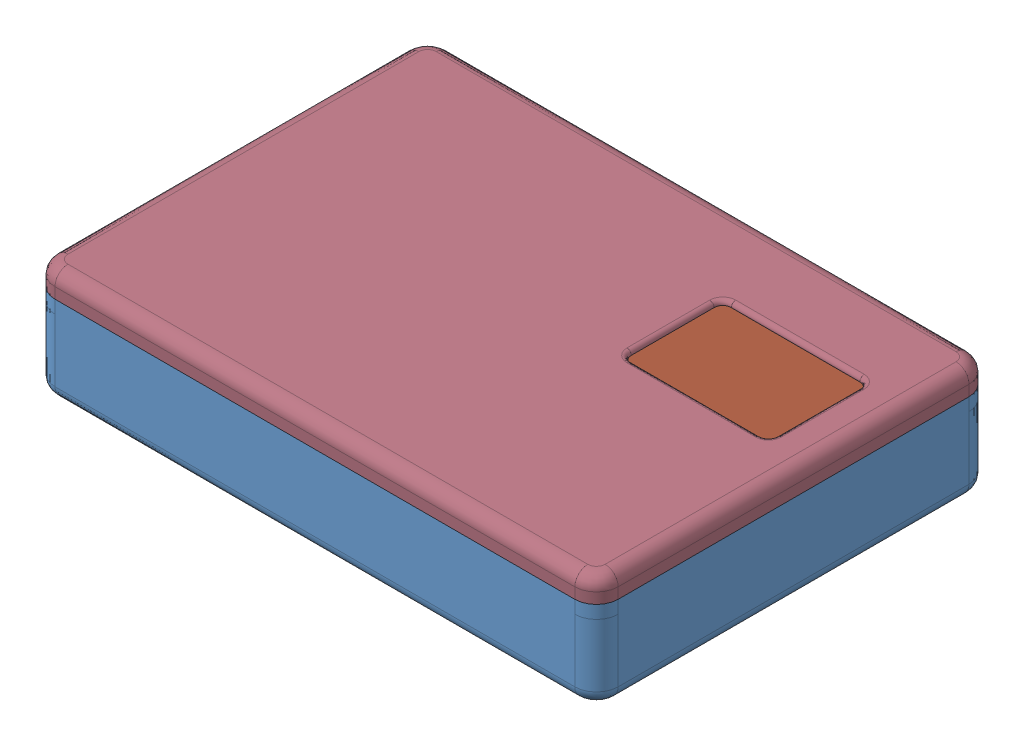
SolidWorks assembly Assembly, configuration Default. Lengths in mm.
Overall size (130.12 26 91.3).
515 component instances, 105 part files, 22 mates.
Components (placement in the parent):
- Part1-1: Part1 [Default] at (-77.6648 36.0917 68.8448) size (130 22.5 91)
- PCB1_2.step-5: PCB1_2.step [Default] at (-142.0534 45.002 144.8645) x (1 0 -0.000465) z (0 1 0) size (68.54 35.94 11.54)
  - Board.step-1: Board.step [Default] at origin size (68.2 35.94 0.41)
    - Open CASCADE STEP translator 7.5 1.1.1.step-1: Open CASCADE STEP translator 7.5 1.1.1.step [Default] at (0 0 -0.4104) size (68.2 35.94 0.41)
  - D6.step-1: D6.step [Default] at origin size (1.3 2.68 1.15)
    - 6259387344.step-1: 6259387344.step [Default] at (99.314 45.339 0) x (0 1 0) z (0 0 1) size (2.67 1.3 1.15)
      - Body.step-1: Body.step [Default] at origin size (1.78 1.3 1.02)
      - FilletPinL.step-1: FilletPinL.step [Default] at origin size (0.45 0.3 0.62)
      - FilletPinR.step-1: FilletPinR.step [Default] at origin size (0.45 0.3 0.62)
  - D5.step-1: D5.step [Default] at origin size (1.3 2.68 1.15)
    - 6259387344.step-1: 6259387344.step [Default] at (97.409 45.466 0) x (0 1 0) z (0 0 1) size (2.67 1.3 1.15)
      - Body.step-1: Body.step [Default] at origin size (1.78 1.3 1.02)
      - FilletPinL.step-1: FilletPinL.step [Default] at origin size (0.45 0.3 0.62)
      - FilletPinR.step-1: FilletPinR.step [Default] at origin size (0.45 0.3 0.62)
  - D4.step-1: D4.step [Default] at origin size (1.3 2.68 1.15)
    - 6259387344.step-1: 6259387344.step [Default] at (75.692 48.387 -0.4104) x (0 -1 0) z (0 0 -1) size (2.67 1.3 1.15)
      - Body.step-1: Body.step [Default] at origin size (1.78 1.3 1.02)
      - FilletPinL.step-1: FilletPinL.step [Default] at origin size (0.45 0.3 0.62)
      - FilletPinR.step-1: FilletPinR.step [Default] at origin size (0.45 0.3 0.62)
  - D3.step-1: D3.step [Default] at origin size (1.3 2.68 1.15)
    - 6259387344.step-1: 6259387344.step [Default] at (75.692 54.356 -0.4104) x (0 -1 0) z (0 0 -1) size (2.67 1.3 1.15)
      - Body.step-1: Body.step [Default] at origin size (1.78 1.3 1.02)
      - FilletPinL.step-1: FilletPinL.step [Default] at origin size (0.45 0.3 0.62)
      - FilletPinR.step-1: FilletPinR.step [Default] at origin size (0.45 0.3 0.62)
  - J3.step-1: J3.step [Default] at origin size (4.01 2 8)
    - Conn_Harwin_M22-2510205_eec.step-1: Conn_Harwin_M22-2510205_eec.step [Default] at (82.931 60.071 0) x (-1 0 0) z (0 0 1) size (4 2 8)
      - Body-0.step-1: Body-0.step [Default] at (-1 0 0.75) x (1 0 0) z (0 -1 0) size (2 1.5 2)
      - Leads.step-1: Leads.step [Default] at (-1 0 0.5) x (-1 0 0) z (0 1 0) size (0.5 8 0.5)
      - Body-0.step-2: Body-0.step [Default] at (1 0 0.75) x (-1 0 0) z (0 1 0) size (2 1.5 2)
      - Leads.step-2: Leads.step [Default] at (1 0 0.5) x (-1 0 0) z (0 1 0) size (0.5 8 0.5)
  - JP3.step-1: JP3.step [Default] at origin size (7.62 2.54 11.54)
    - 61300311121.step-1: 61300311121.step [Default] at (106.0449 39.6239 1.3) x (-1 0 0) z (0 1 0) size (7.62 11.54 2.54)
      - 61300311121-1.step-1: 61300311121-1.step [Default] at origin size (7.62 2.54 2.54)
      - 6130xx11121_PIN.step-1: 6130xx11121_PIN.step [Default] at (-2.54 1.5 0) x (1 0 0) z (0 -1 0) size (0.64 0.64 11.54)
      - 6130xx11121_PIN.step-2: 6130xx11121_PIN.step [Default] at (0 1.5 0) x (1 0 0) z (0 -1 0) size (0.64 0.64 11.54)
      - 6130xx11121_PIN.step-3: 6130xx11121_PIN.step [Default] at (2.54 1.5 0) x (1 0 0) z (0 -1 0) size (0.64 0.64 11.54)
  - R3.step-1: R3.step [Default] at origin size (1.7 0.9 0.55)
    - 6262523328.step-1: 6262523328.step [Default] at (120.381 50.673 0) size (1.2 0.9 0.55)
      - Extruded.step-1: Extruded.step [Default] at origin size (1.2 0.9 0.55)
    - 6262523568.step-1: 6262523568.step [Default] at (119.656 50.673 0) size (0.25 0.9 0.55)
      - Extruded-2.step-1: Extruded-2.step [Default] at origin size (0.25 0.9 0.55)
    - 6262523568.step-2: 6262523568.step [Default] at (121.106 50.673 0) size (0.25 0.9 0.55)
      - Extruded-2.step-1: Extruded-2.step [Default] at origin size (0.25 0.9 0.55)
  - RS1.step-1: RS1.step [Default] at origin size (2.23 3.49 1.16)
    - 6259386784.step-1: 6259386784.step [Default] at (67.945 51.308 -0.4104) x (0 1 0) z (0 0 -1) size (3.49 2.23 1.16)
      - term1.step-1: term1.step [Default] at (-1.6 -0.8 0) size (0.6 1.6 0.65)
      - term2.step-1: term2.step [Default] at (1 -0.8 0) size (0.6 1.6 0.65)
      - Body.step-1: Body.step [Default] at (-1 -0.784 0.0065) size (1.78 1.3 1.02)
  - RNTC1.step-1: RNTC1.step [Default] at origin size (1.6 0.8 0.55)
    - Res_Yageo_RC0603FR-07100KL_eec.step-1: Res_Yageo_RC0603FR-07100KL_eec.step [Default] at (106.4677 42.672 0) x (-1 0 0) z (0 0 1) size (1.6 0.8 0.55)
      - 1.step-1: 1.step [Default] at origin size (1.1 0.8 0.05)
      - 2.step-1: 2.step [Default] at origin size (1.5 0.8 0.45)
      - 3.step-1: 3.step [Default] at origin size (1.6 0.8 0.55)
      - Yageo Logo.step-1: Yageo Logo.step [Default] at (-1.8829 0.0903 0.5401) size (0.34 0.08 0.01)
  - R5.step-1: R5.step [Default] at origin size (1.6 0.8 0.55)
    - 6259379744.step-1: 6259379744.step [Default] at (80.379 48.006 0) x (-1 0 0) z (0 0 1) size (1.6 0.8 0.55)
      - term1-3.step-1: term1-3.step [Default] at (-0.8 -0.4 0) size (0.25 0.8 0.55)
      - term2-4.step-1: term2-4.step [Default] at (0.55 -0.4 0) size (0.25 0.8 0.55)
      - body-5.step-1: body-5.step [Default] at (-0.55 -0.392 0.0055) size (1.1 0.78 0.54)
  - R32.step-1: R32.step [Default] at origin size (2.5 5 0.55)
    - 6151998672.step-1: 6151998672.step [Default] at (98.688 58.674 0) size (2.5 5 0.55)
      - solidBody.step-1: solidBody.step [Default] at origin size (2.4 5 0.45)
      - Terminal.step-1: Terminal.step [Default] at origin size (2.5 5 0.54)
      - solidTop.step-1: solidTop.step [Default] at origin size (1.8 4.9 0.05)
  - R31.step-1: R31.step [Default] at origin size (1.6 0.8 0.55)
    - 6259379744.step-1: 6259379744.step [Default] at (102.87 44.069 0) x (-1 0 0) z (0 0 1) size (1.6 0.8 0.55)
      - term1-3.step-1: term1-3.step [Default] at (-0.8 -0.4 0) size (0.25 0.8 0.55)
      - term2-4.step-1: term2-4.step [Default] at (0.55 -0.4 0) size (0.25 0.8 0.55)
      - body-5.step-1: body-5.step [Default] at (-0.55 -0.392 0.0055) size (1.1 0.78 0.54)
  - R30.step-1: R30.step [Default] at origin size (0.9 1.7 0.55)
    - 6262524208.step-1: 6262524208.step [Default] at (103.124 48.002 0) size (0.9 1.2 0.55)
      - Extruded-6.step-1: Extruded-6.step [Default] at origin size (0.9 1.2 0.55)
    - 6262524048.step-1: 6262524048.step [Default] at (103.124 47.277 0) size (0.9 0.25 0.55)
      - Extruded-7.step-1: Extruded-7.step [Default] at origin size (0.9 0.25 0.55)
    - 6262524048.step-2: 6262524048.step [Default] at (103.124 48.727 0) size (0.9 0.25 0.55)
      - Extruded-7.step-1: Extruded-7.step [Default] at origin size (0.9 0.25 0.55)
  - R29.step-1: R29.step [Default] at origin size (0.8 1.6 0.55)
    - 6259384304.step-1: 6259384304.step [Default] at (111.252 42.168 0) x (0 1 0) z (0 0 1) size (1.6 0.8 0.55)
      - term1-8.step-1: term1-8.step [Default] at (-0.8 -0.4 0) size (0.25 0.8 0.55)
      - term2-9.step-1: term2-9.step [Default] at (0.55 -0.4 0) size (0.25 0.8 0.55)
      - body-10.step-1: body-10.step [Default] at (-0.55 -0.392 0.0055) size (1.1 0.78 0.54)
  - R27.step-1: R27.step [Default] at origin size (0.8 1.6 0.55)
    - 6259384304.step-1: 6259384304.step [Default] at (106.426 45.428 0) x (0 1 0) z (0 0 1) size (1.6 0.8 0.55)
      - term1-8.step-1: term1-8.step [Default] at (-0.8 -0.4 0) size (0.25 0.8 0.55)
      - term2-9.step-1: term2-9.step [Default] at (0.55 -0.4 0) size (0.25 0.8 0.55)
      - body-10.step-1: body-10.step [Default] at (-0.55 -0.392 0.0055) size (1.1 0.78 0.54)
  - R26.step-1: R26.step [Default] at origin size (0.9 1.7 0.55)
    - 6262524208.step-1: 6262524208.step [Default] at (107.823 45.72 0) size (0.9 1.2 0.55)
      - Extruded-6.step-1: Extruded-6.step [Default] at origin size (0.9 1.2 0.55)
    - 6262524048.step-1: 6262524048.step [Default] at (107.823 44.995 0) size (0.9 0.25 0.55)
      - Extruded-7.step-1: Extruded-7.step [Default] at origin size (0.9 0.25 0.55)
    - 6262524048.step-2: 6262524048.step [Default] at (107.823 46.445 0) size (0.9 0.25 0.55)
      - Extruded-7.step-1: Extruded-7.step [Default] at origin size (0.9 0.25 0.55)
  - R25.step-1: R25.step [Default] at origin size (0.8 1.6 0.55)
    - 6259384304.step-1: 6259384304.step [Default] at (101.854 47.752 0) x (0 1 0) z (0 0 1) size (1.6 0.8 0.55)
      - term1-8.step-1: term1-8.step [Default] at (-0.8 -0.4 0) size (0.25 0.8 0.55)
      - term2-9.step-1: term2-9.step [Default] at (0.55 -0.4 0) size (0.25 0.8 0.55)
      - body-10.step-1: body-10.step [Default] at (-0.55 -0.392 0.0055) size (1.1 0.78 0.54)
  - R24.step-1: R24.step [Default] at origin size (1.6 0.8 0.55)
    - 6151993232.step-1: 6151993232.step [Default] at (94.615 46.609 0) size (1.6 0.8 0.55)
      - term1-11.step-1: term1-11.step [Default] at (-0.8 -0.4 0) size (0.25 0.8 0.55)
      - term2-12.step-1: term2-12.step [Default] at (0.55 -0.4 0) size (0.25 0.8 0.55)
      - body-13.step-1: body-13.step [Default] at (-0.55 -0.392 0.0055) size (1.1 0.78 0.54)
  - R23.step-1: R23.step [Default] at origin size (1.6 0.8 0.55)
    - 6259379744.step-1: 6259379744.step [Default] at (80.379 46.228 0) x (-1 0 0) z (0 0 1) size (1.6 0.8 0.55)
      - term1-3.step-1: term1-3.step [Default] at (-0.8 -0.4 0) size (0.25 0.8 0.55)
      - term2-4.step-1: term2-4.step [Default] at (0.55 -0.4 0) size (0.25 0.8 0.55)
      - body-5.step-1: body-5.step [Default] at (-0.55 -0.392 0.0055) size (1.1 0.78 0.54)
  - R22.step-1: R22.step [Default] at origin size (1.7 0.9 0.55)
    - 6262523568.step-1: 6262523568.step [Default] at (107.659 48.387 0) size (0.25 0.9 0.55)
      - Extruded-2.step-1: Extruded-2.step [Default] at origin size (0.25 0.9 0.55)
    - 6262523568.step-2: 6262523568.step [Default] at (106.209 48.387 0) size (0.25 0.9 0.55)
      - Extruded-2.step-1: Extruded-2.step [Default] at origin size (0.25 0.9 0.55)
    - 6262523328.step-1: 6262523328.step [Default] at (106.934 48.387 0) size (1.2 0.9 0.55)
      - Extruded.step-1: Extruded.step [Default] at origin size (1.2 0.9 0.55)
  - R21.step-1: R21.step [Default] at origin size (0.9 1.7 0.55)
    - 6262524208.step-1: 6262524208.step [Default] at (109.474 42.418 0) size (0.9 1.2 0.55)
      - Extruded-6.step-1: Extruded-6.step [Default] at origin size (0.9 1.2 0.55)
    - 6262524048.step-1: 6262524048.step [Default] at (109.474 43.143 0) size (0.9 0.25 0.55)
      - Extruded-7.step-1: Extruded-7.step [Default] at origin size (0.9 0.25 0.55)
    - 6262524048.step-2: 6262524048.step [Default] at (109.474 41.693 0) size (0.9 0.25 0.55)
      - Extruded-7.step-1: Extruded-7.step [Default] at origin size (0.9 0.25 0.55)
  - R20.step-1: R20.step [Default] at origin size (1.6 0.8 0.55)
    - 6259388464.step-1: 6259388464.step [Default] at (94.615 48.006 0) x (1 0 0) z (0 0 1) size (1.6 0.8 0.55)
      - term1-14.step-1: term1-14.step [Default] at (-0.8 -0.4 0) size (0.25 0.8 0.55)
      - term2-15.step-1: term2-15.step [Default] at (0.55 -0.4 0) size (0.25 0.8 0.55)
      - body-16.step-1: body-16.step [Default] at (-0.55 -0.392 0.0055) size (1.1 0.78 0.54)
  - R19.step-1: R19.step [Default] at origin size (0.8 1.6 0.55)
    - 6259384304.step-1: 6259384304.step [Default] at (104.648 47.752 0) x (0 1 0) z (0 0 1) size (1.6 0.8 0.55)
      - term1-8.step-1: term1-8.step [Default] at (-0.8 -0.4 0) size (0.25 0.8 0.55)
      - term2-9.step-1: term2-9.step [Default] at (0.55 -0.4 0) size (0.25 0.8 0.55)
      - body-10.step-1: body-10.step [Default] at (-0.55 -0.392 0.0055) size (1.1 0.78 0.54)
  - R18.step-1: R18.step [Default] at origin size (1.7 0.9 0.55)
    - 6262523328.step-1: 6262523328.step [Default] at (94.615 49.276 0) size (1.2 0.9 0.55)
      - Extruded.step-1: Extruded.step [Default] at origin size (1.2 0.9 0.55)
    - 6262523568.step-1: 6262523568.step [Default] at (93.89 49.276 0) size (0.25 0.9 0.55)
      - Extruded-2.step-1: Extruded-2.step [Default] at origin size (0.25 0.9 0.55)
    - 6262523568.step-2: 6262523568.step [Default] at (95.34 49.276 0) size (0.25 0.9 0.55)
      - Extruded-2.step-1: Extruded-2.step [Default] at origin size (0.25 0.9 0.55)
  - R17.step-1: R17.step [Default] at origin size (1.6 0.8 0.55)
    - Res_Yageo_RC0603FR-07100KL_eec.step-1: Res_Yageo_RC0603FR-07100KL_eec.step [Default] at (94.615 50.8 0) size (1.6 0.8 0.55)
      - 1.step-1: 1.step [Default] at origin size (1.1 0.8 0.05)
      - 2.step-1: 2.step [Default] at origin size (1.5 0.8 0.45)
      - 3.step-1: 3.step [Default] at origin size (1.6 0.8 0.55)
      - Yageo Logo.step-1: Yageo Logo.step [Default] at (-1.8829 0.0903 0.5401) size (0.34 0.08 0.01)
  - R16.step-1: R16.step [Default] at origin size (1.6 0.8 0.55)
    - 6259379744.step-1: 6259379744.step [Default] at (115.443 54.102 0) x (-1 0 0) z (0 0 1) size (1.6 0.8 0.55)
      - term1-3.step-1: term1-3.step [Default] at (-0.8 -0.4 0) size (0.25 0.8 0.55)
      - term2-4.step-1: term2-4.step [Default] at (0.55 -0.4 0) size (0.25 0.8 0.55)
      - body-5.step-1: body-5.step [Default] at (-0.55 -0.392 0.0055) size (1.1 0.78 0.54)
  - R15.step-1: R15.step [Default] at origin size (2.5 5 0.55)
    - 6151998672.step-1: 6151998672.step [Default] at (94.488 58.547 0) size (2.5 5 0.55)
      - solidBody.step-1: solidBody.step [Default] at origin size (2.4 5 0.45)
      - Terminal.step-1: Terminal.step [Default] at origin size (2.5 5 0.54)
      - solidTop.step-1: solidTop.step [Default] at origin size (1.8 4.9 0.05)
  - R14.step-1: R14.step [Default] at origin size (1.7 0.9 0.55)
    - 6262523568.step-1: 6262523568.step [Default] at (85.561 51.943 0) size (0.25 0.9 0.55)
      - Extruded-2.step-1: Extruded-2.step [Default] at origin size (0.25 0.9 0.55)
    - 6262523568.step-2: 6262523568.step [Default] at (84.111 51.943 0) size (0.25 0.9 0.55)
      - Extruded-2.step-1: Extruded-2.step [Default] at origin size (0.25 0.9 0.55)
    - 6262523328.step-1: 6262523328.step [Default] at (84.836 51.943 0) size (1.2 0.9 0.55)
      - Extruded.step-1: Extruded.step [Default] at origin size (1.2 0.9 0.55)
  - R13.step-1: R13.step [Default] at origin size (2.5 5 0.55)
    - 6151998672.step-1: 6151998672.step [Default] at (126.365 58.928 0) size (2.5 5 0.55)
      - solidBody.step-1: solidBody.step [Default] at origin size (2.4 5 0.45)
      - Terminal.step-1: Terminal.step [Default] at origin size (2.5 5 0.54)
      - solidTop.step-1: solidTop.step [Default] at origin size (1.8 4.9 0.05)
  - R12.step-1: R12.step [Default] at origin size (2.5 5 0.55)
    - 6151998672.step-1: 6151998672.step [Default] at (122.174 58.928 0) size (2.5 5 0.55)
      - solidBody.step-1: solidBody.step [Default] at origin size (2.4 5 0.45)
      - Terminal.step-1: Terminal.step [Default] at origin size (2.5 5 0.54)
      - solidTop.step-1: solidTop.step [Default] at origin size (1.8 4.9 0.05)
  - R11.step-1: R11.step [Default] at origin size (1.6 0.8 0.55)
    - 6259379744.step-1: 6259379744.step [Default] at (94.5879 54.102 0) x (-1 0 0) z (0 0 1) size (1.6 0.8 0.55)
      - term1-3.step-1: term1-3.step [Default] at (-0.8 -0.4 0) size (0.25 0.8 0.55)
      - term2-4.step-1: term2-4.step [Default] at (0.55 -0.4 0) size (0.25 0.8 0.55)
      - body-5.step-1: body-5.step [Default] at (-0.55 -0.392 0.0055) size (1.1 0.78 0.54)
  - R10.step-1: R10.step [Default] at origin size (1.6 0.8 0.55)
    - 6259379744.step-1: 6259379744.step [Default] at (94.5879 52.451 0) x (-1 0 0) z (0 0 1) size (1.6 0.8 0.55)
      - term1-3.step-1: term1-3.step [Default] at (-0.8 -0.4 0) size (0.25 0.8 0.55)
      - term2-4.step-1: term2-4.step [Default] at (0.55 -0.4 0) size (0.25 0.8 0.55)
      - body-5.step-1: body-5.step [Default] at (-0.55 -0.392 0.0055) size (1.1 0.78 0.54)
  - R9.step-1: R9.step [Default] at origin size (1.6 0.8 0.55)
    - 6151993232.step-1: 6151993232.step [Default] at (115.443 55.753 0) size (1.6 0.8 0.55)
      - term1-11.step-1: term1-11.step [Default] at (-0.8 -0.4 0) size (0.25 0.8 0.55)
      - term2-12.step-1: term2-12.step [Default] at (0.55 -0.4 0) size (0.25 0.8 0.55)
      - body-13.step-1: body-13.step [Default] at (-0.55 -0.392 0.0055) size (1.1 0.78 0.54)
  - R8.step-1: R8.step [Default] at origin size (0.8 1.6 0.55)
    - 6259393184.step-1: 6259393184.step [Default] at (118.237 62.23 0) x (0 -1 0) z (0 0 1) size (1.6 0.8 0.55)
      - term1-17.step-1: term1-17.step [Default] at (-0.8 -0.4 0) size (0.25 0.8 0.55)
      - term2-18.step-1: term2-18.step [Default] at (0.55 -0.4 0) size (0.25 0.8 0.55)
      - body-19.step-1: body-19.step [Default] at (-0.55 -0.392 0.0055) size (1.1 0.78 0.54)
  - R7.step-1: R7.step [Default] at origin size (0.8 1.6 0.55)
    - 6259384304.step-1: 6259384304.step [Default] at (109.728 62.268 0) x (0 1 0) z (0 0 1) size (1.6 0.8 0.55)
      - term1-8.step-1: term1-8.step [Default] at (-0.8 -0.4 0) size (0.25 0.8 0.55)
      - term2-9.step-1: term2-9.step [Default] at (0.55 -0.4 0) size (0.25 0.8 0.55)
      - body-10.step-1: body-10.step [Default] at (-0.55 -0.392 0.0055) size (1.1 0.78 0.54)
  - R6.step-1: R6.step [Default] at origin size (0.8 1.6 0.55)
    - 6259393184.step-1: 6259393184.step [Default] at (90.551 48.73 0) x (0 -1 0) z (0 0 1) size (1.6 0.8 0.55)
      - term1-17.step-1: term1-17.step [Default] at (-0.8 -0.4 0) size (0.25 0.8 0.55)
      - term2-18.step-1: term2-18.step [Default] at (0.55 -0.4 0) size (0.25 0.8 0.55)
      - body-19.step-1: body-19.step [Default] at (-0.55 -0.392 0.0055) size (1.1 0.78 0.54)
  - R4.step-1: R4.step [Default] at origin size (1.7 0.9 0.55)
    - 6262523568.step-1: 6262523568.step [Default] at (125.17 46.101 0) size (0.25 0.9 0.55)
      - Extruded-2.step-1: Extruded-2.step [Default] at origin size (0.25 0.9 0.55)
    - 6262523568.step-2: 6262523568.step [Default] at (123.72 46.101 0) size (0.25 0.9 0.55)
      - Extruded-2.step-1: Extruded-2.step [Default] at origin size (0.25 0.9 0.55)
    - 6262523328.step-1: 6262523328.step [Default] at (124.445 46.101 0) size (1.2 0.9 0.55)
      - Extruded.step-1: Extruded.step [Default] at origin size (1.2 0.9 0.55)
  - R2.step-1: R2.step [Default] at origin size (1.6 0.8 0.55)
    - 6259379744.step-1: 6259379744.step [Default] at (124.549 47.752 0) x (-1 0 0) z (0 0 1) size (1.6 0.8 0.55)
      - term1-3.step-1: term1-3.step [Default] at (-0.8 -0.4 0) size (0.25 0.8 0.55)
      - term2-4.step-1: term2-4.step [Default] at (0.55 -0.4 0) size (0.25 0.8 0.55)
      - body-5.step-1: body-5.step [Default] at (-0.55 -0.392 0.0055) size (1.1 0.78 0.54)
  - R1.step-1: R1.step [Default] at origin size (0.8 1.6 0.55)
    - 6259384304.step-1: 6259384304.step [Default] at (118.872 53.213 0) x (0 1 0) z (0 0 1) size (1.6 0.8 0.55)
      - term1-8.step-1: term1-8.step [Default] at (-0.8 -0.4 0) size (0.25 0.8 0.55)
      - term2-9.step-1: term2-9.step [Default] at (0.55 -0.4 0) size (0.25 0.8 0.55)
      - body-10.step-1: body-10.step [Default] at (-0.55 -0.392 0.0055) size (1.1 0.78 0.54)
  - P2.step-1: P2.step [Default] at origin size (12.7 2.54 11.54)
    - 61300511121.step-1: 61300511121.step [Default] at (94.2339 39.7509 1.3) x (-1 0 0) z (0 1 0) size (12.7 11.54 2.54)
      - 6130xx11121_PIN-20.step-1: 6130xx11121_PIN-20.step [Default] at (-5.08 1.5 0) x (1 0 0) z (0 -1 0) size (0.64 0.64 11.54)
      - 6130xx11121_PIN-20.step-2: 6130xx11121_PIN-20.step [Default] at (-2.54 1.5 0) x (1 0 0) z (0 -1 0) size (0.64 0.64 11.54)
      - 6130xx11121_PIN-20.step-3: 6130xx11121_PIN-20.step [Default] at (0 1.5 0) x (1 0 0) z (0 -1 0) size (0.64 0.64 11.54)
      - 6130xx11121_PIN-20.step-4: 6130xx11121_PIN-20.step [Default] at (2.54 1.5 0) x (1 0 0) z (0 -1 0) size (0.64 0.64 11.54)
      - 6130xx11121_PIN-20.step-5: 6130xx11121_PIN-20.step [Default] at (5.08 1.5 0) x (1 0 0) z (0 -1 0) size (0.64 0.64 11.54)
      - 61300511121-21.step-1: 61300511121-21.step [Default] at origin size (12.7 2.54 2.54)
  - P1.step-1: P1.step [Default] at origin size (10.49 9.2 5.39)
    - 6259392944.step-1: 6259392944.step [Default] at (64.299 51.054 1.59) x (-1 0 0) z (0 0 1) size (10.49 9.2 5.39)
  - M2.step-1: M2.step [Default] at origin size (3.3 3.3 1.06)
    - 6259390624.step-1: 6259390624.step [Default] at (88.799 55.336 0.02) x (-1 0 0) z (0 1 0) size (3.3 1.06 3.3)
  - M1.step-1: M1.step [Default] at origin size (3.3 3.3 1.06)
    - 6259390624.step-1: 6259390624.step [Default] at (84.709 55.246 0.02) x (-1 0 0) z (0 1 0) size (3.3 1.06 3.3)
  - LED1.step-1: LED1.step [Default] at origin size (1 2 0.7)
    - 6259379424.step-1: 6259379424.step [Default] at (110.774 46.833 0.12) x (0 -1 0) z (-1 0 0) size (2 0.7 1)
  - L1.step-1: L1.step [Default] at origin size (4 4 3.1)
    - 6151993152.step-1: 6151993152.step [Default] at (113.919 60.579 0) size (4 4 3.1)
      - Body-22.step-1: Body-22.step [Default] at (0 0 0.1) size (4 4 3)
      - Pins.step-1: Pins.step [Default] at origin size (3.87 3.37 0.1)
  - JP2.step-1: JP2.step [Default] at origin size (7.62 2.54 11.54)
    - 61300311121.step-1: 61300311121.step [Default] at (117.0941 41.5291 1.3) x (1 0 0) z (0 -1 0) size (7.62 11.54 2.54)
      - 61300311121-1.step-1: 61300311121-1.step [Default] at origin size (7.62 2.54 2.54)
      - 6130xx11121_PIN.step-1: 6130xx11121_PIN.step [Default] at (-2.54 1.5 0) x (1 0 0) z (0 -1 0) size (0.64 0.64 11.54)
      - 6130xx11121_PIN.step-2: 6130xx11121_PIN.step [Default] at (0 1.5 0) x (1 0 0) z (0 -1 0) size (0.64 0.64 11.54)
      - 6130xx11121_PIN.step-3: 6130xx11121_PIN.step [Default] at (2.54 1.5 0) x (1 0 0) z (0 -1 0) size (0.64 0.64 11.54)
  - J2.step-1: J2.step [Default] at origin size (2 4.01 8)
    - Conn_Harwin_M22-2510205_eec.step-1: Conn_Harwin_M22-2510205_eec.step [Default] at (128.397 50.53 0) x (0 1 0) z (0 0 1) size (4 2 8)
      - Body-0.step-1: Body-0.step [Default] at (-1 0 0.75) x (1 0 0) z (0 -1 0) size (2 1.5 2)
      - Leads.step-1: Leads.step [Default] at (-1 0 0.5) x (-1 0 0) z (0 1 0) size (0.5 8 0.5)
      - Body-0.step-2: Body-0.step [Default] at (1 0 0.75) x (-1 0 0) z (0 1 0) size (2 1.5 2)
      - Leads.step-2: Leads.step [Default] at (1 0 0.5) x (-1 0 0) z (0 1 0) size (0.5 8 0.5)
  - IC3.step-1: IC3.step [Default] at origin size (2.1 2 1)
    - 6259382224.step-1: 6259382224.step [Default] at (124.46 50.673 0) x (1 0 0) z (0 0 1) size (2.1 2 1)
      - Body-23.step-1: Body-23.step [Default] at origin size (2 2 0.95)
      - ThermalPin.step-1: ThermalPin.step [Default] at (-0.375 -0.675 0) size (0.75 1.35 0.12)
      - PinsArrayLR.step-1: PinsArrayLR.step [Default] at origin size (2.1 1.55 0.12)
  - IC1.step-1: IC1.step [Default] at origin size (4.1 4.1 0.6)
    - 6259389504.step-1: 6259389504.step [Default] at (84.963 44.704 0) x (0 1 0) z (0 0 1) size (4.1 4.1 0.6)
      - Body-24.step-1: Body-24.step [Default] at origin size (4 4 0.55)
      - ThermalPin-25.step-1: ThermalPin-25.step [Default] at (-1.375 -1.375 0) size (2.75 2.75 0.1)
      - PinsArrayLR-26.step-1: PinsArrayLR-26.step [Default] at origin size (4.1 2.74 0.1)
      - PinsArrayTB.step-1: PinsArrayTB.step [Default] at origin size (2.74 4.1 0.1)
  - ETCH1.step-1: ETCH1.step [Default] at origin size (1.6 0.8 0.55)
    - 6259379744.step-1: 6259379744.step [Default] at (98.234 51.689 0) x (-1 0 0) z (0 0 1) size (1.6 0.8 0.55)
      - term1-3.step-1: term1-3.step [Default] at (-0.8 -0.4 0) size (0.25 0.8 0.55)
      - term2-4.step-1: term2-4.step [Default] at (0.55 -0.4 0) size (0.25 0.8 0.55)
      - body-5.step-1: body-5.step [Default] at (-0.55 -0.392 0.0055) size (1.1 0.78 0.54)
  - D2.step-1: D2.step [Default] at origin size (3.65 1.55 1.45)
    - Diode_Diodes_Inc_B0520LW-7-F_eec.step-1: Diode_Diodes_Inc_B0520LW-7-F_eec.step [Default] at (119.38 45.212 0) x (1 0 0) z (0 0 1) size (3.65 1.55 1.45)
      - 1-27.step-1: 1-27.step [Default] at (0 0 0.1) size (2.65 1.55 1.35)
      - 2-28.step-1: 2-28.step [Default] at (0.0059 0.0003 1.352) size (0.15 0.92 0.1)
      - 3-29.step-1: 3-29.step [Default] x (1 0 0) z (0 -1 0) size (3.65 0.6 0.57)
      - Diod Logo.step-1: Diod Logo.step [Default] at (-1.6659 0.0681 1.441) size (0.92 0.23 0.01)
  - D1.step-1: D1.step [Default] at origin size (3.65 1.55 1.45)
    - Diode_Diodes_Inc_B0520LW-7-F_eec.step-1: Diode_Diodes_Inc_B0520LW-7-F_eec.step [Default] at (119.38 47.752 0) x (1 0 0) z (0 0 1) size (3.65 1.55 1.45)
      - 1-27.step-1: 1-27.step [Default] at (0 0 0.1) size (2.65 1.55 1.35)
      - 2-28.step-1: 2-28.step [Default] at (0.0059 0.0003 1.352) size (0.15 0.92 0.1)
      - 3-29.step-1: 3-29.step [Default] x (1 0 0) z (0 -1 0) size (3.65 0.6 0.57)
      - Diod Logo.step-1: Diod Logo.step [Default] at (-1.6659 0.0681 1.441) size (0.92 0.23 0.01)
  - C36.step-1: C36.step [Default] at origin size (1.25 2 1.46)
    - Cap_Murata_GRM21BC71C106KE11L_eec.step-1: Cap_Murata_GRM21BC71C106KE11L_eec.step [Default] at (114.173 46.355 0) x (0 1 0) z (0 0 1) size (2 1.25 1.46)
      - body-30.step-1: body-30.step [Default] x (-1 0 0) z (0 0 1) size (1.1 1.25 1.45)
      - side.step-1: side.step [Default] at (-0.7 0.2667 0) x (-1 0 0) z (0 0 1) size (0.45 1.25 1.45)
      - side.step-2: side.step [Default] at (0.7 0.2667 1.45) x (1 0 0) z (0 0 -1) size (0.45 1.25 1.45)
      - Murata.step-1: Murata.step [Default] at (-0.7353 -0.8898 1.447) size (0.61 0.14 0.01)
  - C34.step-1: C34.step [Default] at origin size (2 1.25 1.45)
    - 6259380704.step-1: 6259380704.step [Default] at (80.264 41.275 0) x (1 0 0) z (0 0 1) size (2 1.25 1.45)
      - Fillet1.step-1: Fillet1.step [Default] at origin size (0.45 1.25 1.45)
      - Fillet2.step-1: Fillet2.step [Default] at origin size (0.45 1.25 1.45)
      - body2.step-1: body2.step [Default] at origin size (1.1 1.22 1.42)
  - C33.step-1: C33.step [Default] at origin size (1.6 0.8 0.87)
    - 6259379824.step-1: 6259379824.step [Default] at (80.509 43.053 0) x (1 0 0) z (0 0 1) size (1.6 0.8 0.87)
      - Fillet1-31.step-1: Fillet1-31.step [Default] at origin size (0.4 0.8 0.87)
      - Fillet2-32.step-1: Fillet2-32.step [Default] at origin size (0.4 0.8 0.87)
      - body2-33.step-1: body2-33.step [Default] at origin size (0.8 0.78 0.85)
  - C32.step-1: C32.step [Default] at origin size (2 1.25 1.45)
    - 6259393024.step-1: 6259393024.step [Default] at (89.8569 43.815 0) x (-1 0 0) z (0 0 1) size (2 1.25 1.45)
      - Fillet1-34.step-1: Fillet1-34.step [Default] at origin size (0.45 1.25 1.45)
      - Fillet2-35.step-1: Fillet2-35.step [Default] at origin size (0.45 1.25 1.45)
      - body2-36.step-1: body2-36.step [Default] at origin size (1.1 1.22 1.42)
  - C31.step-1: C31.step [Default] at origin size (1.6 0.8 0.87)
    - 6259392704.step-1: 6259392704.step [Default] at (80.509 39.116 0) x (-1 0 0) z (0 0 1) size (1.6 0.8 0.87)
      - Fillet1-37.step-1: Fillet1-37.step [Default] at origin size (0.4 0.8 0.87)
      - Fillet2-38.step-1: Fillet2-38.step [Default] at origin size (0.4 0.8 0.87)
      - body2-39.step-1: body2-39.step [Default] at origin size (0.8 0.78 0.85)
  - C30.step-1: C30.step [Default] at origin size (1.6 0.8 0.87)
    - 6259379824.step-1: 6259379824.step [Default] at (80.509 44.704 0) x (1 0 0) z (0 0 1) size (1.6 0.8 0.87)
      - Fillet1-31.step-1: Fillet1-31.step [Default] at origin size (0.4 0.8 0.87)
      - Fillet2-32.step-1: Fillet2-32.step [Default] at origin size (0.4 0.8 0.87)
      - body2-33.step-1: body2-33.step [Default] at origin size (0.8 0.78 0.85)
  - C29.step-1: C29.step [Default] at origin size (1.25 2 1.46)
    - Cap_Murata_GRM21BC71C106KE11L_eec.step-1: Cap_Murata_GRM21BC71C106KE11L_eec.step [Default] at (115.824 51.181 0) x (0 1 0) z (0 0 1) size (2 1.25 1.46)
      - body-30.step-1: body-30.step [Default] x (-1 0 0) z (0 0 1) size (1.1 1.25 1.45)
      - side.step-1: side.step [Default] at (-0.7 0.2667 0) x (-1 0 0) z (0 0 1) size (0.45 1.25 1.45)
      - side.step-2: side.step [Default] at (0.7 0.2667 1.45) x (1 0 0) z (0 0 -1) size (0.45 1.25 1.45)
      - Murata.step-1: Murata.step [Default] at (-0.7353 -0.8898 1.447) size (0.61 0.14 0.01)
  - C28.step-1: C28.step [Default] at origin size (1.25 2 1.46)
    - Cap_Murata_GRM21BC71C106KE11L_eec.step-1: Cap_Murata_GRM21BC71C106KE11L_eec.step [Default] at (113.284 51.181 0) x (0 1 0) z (0 0 1) size (2 1.25 1.46)
      - body-30.step-1: body-30.step [Default] x (-1 0 0) z (0 0 1) size (1.1 1.25 1.45)
      - side.step-1: side.step [Default] at (-0.7 0.2667 0) x (-1 0 0) z (0 0 1) size (0.45 1.25 1.45)
      - side.step-2: side.step [Default] at (0.7 0.2667 1.45) x (1 0 0) z (0 0 -1) size (0.45 1.25 1.45)
      - Murata.step-1: Murata.step [Default] at (-0.7353 -0.8898 1.447) size (0.61 0.14 0.01)
  - C27.step-1: C27.step [Default] at origin size (1.25 2 1.46)
    - Cap_Murata_GRM21BC71C106KE11L_eec.step-1: Cap_Murata_GRM21BC71C106KE11L_eec.step [Default] at (110.617 51.181 0) x (0 1 0) z (0 0 1) size (2 1.25 1.46)
      - body-30.step-1: body-30.step [Default] x (-1 0 0) z (0 0 1) size (1.1 1.25 1.45)
      - side.step-1: side.step [Default] at (-0.7 0.2667 0) x (-1 0 0) z (0 0 1) size (0.45 1.25 1.45)
      - side.step-2: side.step [Default] at (0.7 0.2667 1.45) x (1 0 0) z (0 0 -1) size (0.45 1.25 1.45)
      - Murata.step-1: Murata.step [Default] at (-0.7353 -0.8898 1.447) size (0.61 0.14 0.01)
  - C22.step-1: C22.step [Default] at origin size (1.25 2 1.4)
    - Cap_Murata_GRM21BC81C106KA73L_eec.step-1: Cap_Murata_GRM21BC81C106KA73L_eec.step [Default] at (87.884 49.2561 0) x (0 1 0) z (0 0 1) size (2 1.25 1.4)
      - 1-40.step-1: 1-40.step [Default] at origin size (2 1.25 1.4)
      - 2-41.step-1: 2-41.step [Default] at (0 0 0.01) size (1.98 1.23 1.38)
      - Murata Logo 3.step-1: Murata Logo 3.step [Default] at (-0.1814 -0.5957 1.2901) size (0.53 0.12 0.1)
  - C21.step-1: C21.step [Default] at origin size (2 1.25 1.4)
    - Cap_Murata_GRM21BC81C106KA73L_eec.step-1: Cap_Murata_GRM21BC81C106KA73L_eec.step [Default] at (102.7788 62.357 0) x (-1 0 0) z (0 0 1) size (2 1.25 1.4)
      - 1-40.step-1: 1-40.step [Default] at origin size (2 1.25 1.4)
